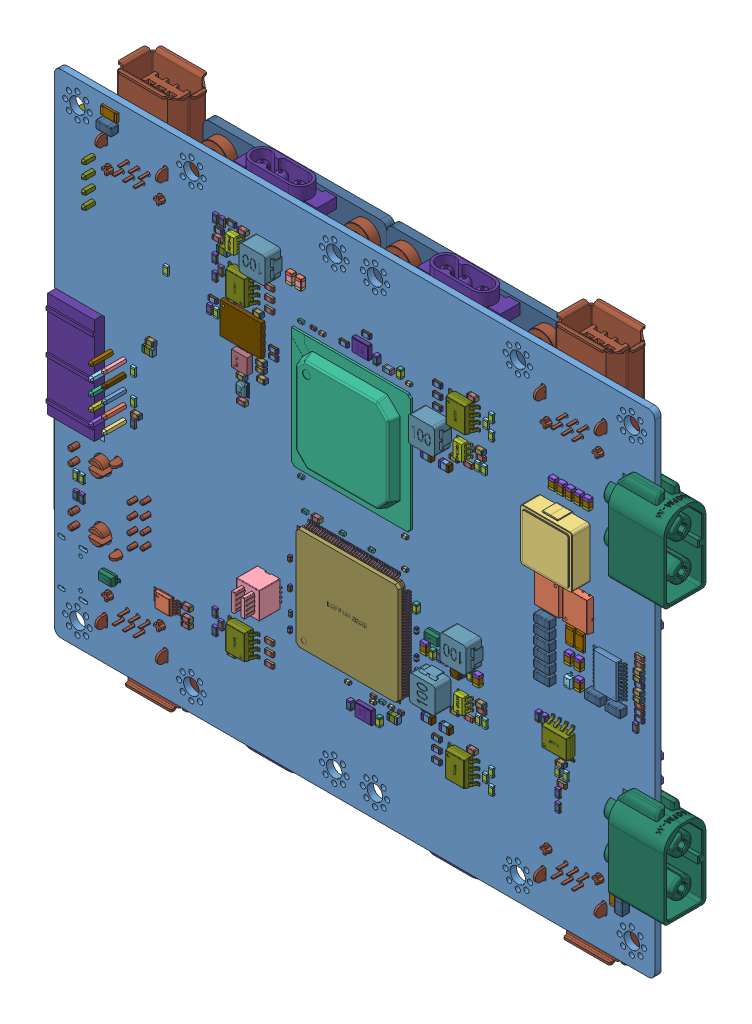
SolidWorks assembly Mother  Board, configuration 默认. Lengths in mm. (continued)
Components (placement in the parent): (continued)
- Mother  Board.step-1: Mother  Board.step [默认] at origin size (122.6 102.08 21) (continued)
  - C1_D4.step-1: C1_D4.step [默认] at origin size (1.6 0.8 0.8) (continued)
    - 5993854224.step-1: 5993854224.step [默认] at (76.6661 75.9461 0) x (1 0 0) z (0 0 1) size (1.6 0.8 0.8) (continued)
      - Terminal-17.step-1: Terminal-17.step [默认] at (-0.8 -0.4 0) size (1.6 0.8 0.8) (continued)
        - Open_CASCADE_STEP_translator_6.8_47.1.2-61.step-1: Open_CASCADE_STEP_translator_6.8_47.1.2-61.step [默认] at origin size (0.3 0.8 0.8)
      - Mid_Body-8.step-1: Mid_Body-8.step [默认] at (-0.8 -0.4 0) size (1 0.8 0.8)
        - Open_CASCADE_STEP_translator_6.8_47.2.1-62.step-1: Open_CASCADE_STEP_translator_6.8_47.2.1-62.step [默认] at origin size (1 0.8 0.8)
  - C1_D3.step-1: C1_D3.step [默认] at origin size (1.6 0.8 0.8)
    - 5993853264.step-1: 5993853264.step [默认] at (30.3949 69.2149 0) x (-1 0 0) z (0 0 1) size (1.6 0.8 0.8)
      - Terminal-6.step-1: Terminal-6.step [默认] at (-0.8 -0.4 0) size (1.6 0.8 0.8)
        - Open_CASCADE_STEP_translator_6.8_47.1.1-10.step-1: Open_CASCADE_STEP_translator_6.8_47.1.1-10.step [默认] at origin size (0.3 0.8 0.8)
        - Open_CASCADE_STEP_translator_6.8_47.1.2-11.step-1: Open_CASCADE_STEP_translator_6.8_47.1.2-11.step [默认] at origin size (0.3 0.8 0.8)
      - Mid_Body-5.step-1: Mid_Body-5.step [默认] at (-0.8 -0.4 0) size (1 0.8 0.8)
        - Open_CASCADE_STEP_translator_6.8_47.2.1-12.step-1: Open_CASCADE_STEP_translator_6.8_47.2.1-12.step [默认] at origin size (1 0.8 0.8)
  - C1_D2.step-1: C1_D2.step [默认] at origin size (1.6 0.8 0.8)
    - 5993854224.step-1: 5993854224.step [默认] at (76.5811 16.8911 0) x (1 0 0) z (0 0 1) size (1.6 0.8 0.8)
      - Terminal-17.step-1: Terminal-17.step [默认] at (-0.8 -0.4 0) size (1.6 0.8 0.8)
        - Open_CASCADE_STEP_translator_6.8_47.1.1-60.step-1: Open_CASCADE_STEP_translator_6.8_47.1.1-60.step [默认] at origin size (0.3 0.8 0.8)
        - Open_CASCADE_STEP_translator_6.8_47.1.2-61.step-1: Open_CASCADE_STEP_translator_6.8_47.1.2-61.step [默认] at origin size (0.3 0.8 0.8)
      - Mid_Body-8.step-1: Mid_Body-8.step [默认] at (-0.8 -0.4 0) size (1 0.8 0.8)
        - Open_CASCADE_STEP_translator_6.8_47.2.1-62.step-1: Open_CASCADE_STEP_translator_6.8_47.2.1-62.step [默认] at origin size (1 0.8 0.8)
  - C1_D1.step-1: C1_D1.step [默认] at origin size (1.6 0.8 0.8)
    - 5993853264.step-1: 5993853264.step [默认] at (30.3949 10.0329 0) x (-1 0 0) z (0 0 1) size (1.6 0.8 0.8)
      - Terminal-6.step-1: Terminal-6.step [默认] at (-0.8 -0.4 0) size (1.6 0.8 0.8)
        - Open_CASCADE_STEP_translator_6.8_47.1.1-10.step-1: Open_CASCADE_STEP_translator_6.8_47.1.1-10.step [默认] at origin size (0.3 0.8 0.8)
        - Open_CASCADE_STEP_translator_6.8_47.1.2-11.step-1: Open_CASCADE_STEP_translator_6.8_47.1.2-11.step [默认] at origin size (0.3 0.8 0.8)
      - Mid_Body-5.step-1: Mid_Body-5.step [默认] at (-0.8 -0.4 0) size (1 0.8 0.8)
        - Open_CASCADE_STEP_translator_6.8_47.2.1-12.step-1: Open_CASCADE_STEP_translator_6.8_47.2.1-12.step [默认] at origin size (1 0.8 0.8)
  - Free-Models.step-1: Free-Models.step [默认] at origin size (70.87 98.07 8.62)
    - Driver_Board.step-1: Driver_Board.step [默认] at (49.5407 86.106 -6.2) x (-1 0 0) z (0 0 1) size (35.43 49.03 8.62)
      - Board-1.step-1: Board-1.step [默认] at origin size (35.43 46.99 1.62)
        - Open_CASCADE_STEP_translator_6.8_2.1.1.step-1: Open_CASCADE_STEP_translator_6.8_2.1.1.step [默认] at (0 0 -1.6164) size (35.43 46.99 1.62)
      - R25-1.step-1: R25-1.step [默认] at origin size (0.8 1.6 0.45)
        - 6547515376.step-1: 6547515376.step [默认] at (20.6304 35.5601 0) x (0 1 0) z (0 0 1) size (1.6 0.8 0.45)
          - Terminal-19.step-1: Terminal-19.step [默认] at (-0.8 -0.4 0) size (0.3 0.8 0.45)
            - Open_CASCADE_STEP_translator_6.8_21.2.1-76.step-1: Open_CASCADE_STEP_translator_6.8_21.2.1-76.step [默认] at origin size (0.3 0.8 0.45)
          - Terminal-19.step-2: Terminal-19.step [默认] at (0.8 0.4 0) x (-1 0 0) z (0 0 1) size (0.3 0.8 0.45)
            - Open_CASCADE_STEP_translator_6.8_21.2.1-76.step-1: Open_CASCADE_STEP_translator_6.8_21.2.1-76.step [默认] at origin size (0.3 0.8 0.45)
          - Mid_Body-77.step-1: Mid_Body-77.step [默认] at (-0.8 -0.4 0) size (1.51 0.8 0.36)
          - Mark-78.step-1: Mark-78.step [默认] at (-0.5 -0.4 0.405) size (1 0.8 0.05)
      - R24-1.step-1: R24-1.step [默认] at origin size (1.6 0.8 0.45)
        - 6547516336.step-1: 6547516336.step [默认] at (12.6999 34.9249 0) x (-1 0 0) z (0 0 1) size (1.6 0.8 0.45)
          - Terminal-20.step-1: Terminal-20.step [默认] at (-0.8 -0.4 0) size (0.3 0.8 0.45)
            - Open_CASCADE_STEP_translator_6.8_21.2.1-79.step-1: Open_CASCADE_STEP_translator_6.8_21.2.1-79.step [默认] at origin size (0.3 0.8 0.45)
          - Terminal-20.step-2: Terminal-20.step [默认] at (0.8 0.4 0) x (-1 0 0) z (0 0 1) size (0.3 0.8 0.45)
            - Open_CASCADE_STEP_translator_6.8_21.2.1-79.step-1: Open_CASCADE_STEP_translator_6.8_21.2.1-79.step [默认] at origin size (0.3 0.8 0.45)
          - Mid_Body-80.step-1: Mid_Body-80.step [默认] at (-0.8 -0.4 0) size (1.51 0.8 0.36)
          - Mark-81.step-1: Mark-81.step [默认] at (-0.5 -0.4 0.405) size (1 0.8 0.05)
      - R23-1.step-1: R23-1.step [默认] at origin size (1.6 0.8 0.45)
        - 6547516336.step-1: 6547516336.step [默认] at (5.5879 33.6549 0) x (-1 0 0) z (0 0 1) size (1.6 0.8 0.45)
          - Terminal-20.step-1: Terminal-20.step [默认] at (-0.8 -0.4 0) size (0.3 0.8 0.45)
            - Open_CASCADE_STEP_translator_6.8_21.2.1-79.step-1: Open_CASCADE_STEP_translator_6.8_21.2.1-79.step [默认] at origin size (0.3 0.8 0.45)
          - Terminal-20.step-2: Terminal-20.step [默认] at (0.8 0.4 0) x (-1 0 0) z (0 0 1) size (0.3 0.8 0.45)
            - Open_CASCADE_STEP_translator_6.8_21.2.1-79.step-1: Open_CASCADE_STEP_translator_6.8_21.2.1-79.step [默认] at origin size (0.3 0.8 0.45)
          - Mid_Body-80.step-1: Mid_Body-80.step [默认] at (-0.8 -0.4 0) size (1.51 0.8 0.36)
          - Mark-81.step-1: Mark-81.step [默认] at (-0.5 -0.4 0.405) size (1 0.8 0.05)
      - JP1.step-1: JP1.step [默认] at origin size (16.01 14.49 6.96)
        - User_Library-MR30PW-M.step-1: User_Library-MR30PW-M.step [默认] at (13.7158 -5.9802 2.75) x (1 0 0) z (0 0 1) size (16.01 14.49 6.96)
      - R18-1.step-1: R18-1.step [默认] at origin size (0.8 1.6 0.45)
        - 6547515376.step-1: 6547515376.step [默认] at (22.9869 34.4171 0) x (0 1 0) z (0 0 1) size (1.6 0.8 0.45)
          - Terminal-19.step-1: Terminal-19.step [默认] at (-0.8 -0.4 0) size (0.3 0.8 0.45)
            - Open_CASCADE_STEP_translator_6.8_21.2.1-76.step-1: Open_CASCADE_STEP_translator_6.8_21.2.1-76.step [默认] at origin size (0.3 0.8 0.45)
          - Terminal-19.step-2: Terminal-19.step [默认] at (0.8 0.4 0) x (-1 0 0) z (0 0 1) size (0.3 0.8 0.45)
            - Open_CASCADE_STEP_translator_6.8_21.2.1-76.step-1: Open_CASCADE_STEP_translator_6.8_21.2.1-76.step [默认] at origin size (0.3 0.8 0.45)
          - Mid_Body-77.step-1: Mid_Body-77.step [默认] at (-0.8 -0.4 0) size (1.51 0.8 0.36)
          - Mark-78.step-1: Mark-78.step [默认] at (-0.5 -0.4 0.405) size (1 0.8 0.05)
      - R17-1.step-1: R17-1.step [默认] at origin size (0.8 1.6 0.45)
        - 6547515376.step-1: 6547515376.step [默认] at (21.8663 34.3947 0) x (0 1 0) z (0 0 1) size (1.6 0.8 0.45)
          - Terminal-19.step-1: Terminal-19.step [默认] at (-0.8 -0.4 0) size (0.3 0.8 0.45)
            - Open_CASCADE_STEP_translator_6.8_21.2.1-76.step-1: Open_CASCADE_STEP_translator_6.8_21.2.1-76.step [默认] at origin size (0.3 0.8 0.45)
          - Terminal-19.step-2: Terminal-19.step [默认] at (0.8 0.4 0) x (-1 0 0) z (0 0 1) size (0.3 0.8 0.45)
            - Open_CASCADE_STEP_translator_6.8_21.2.1-76.step-1: Open_CASCADE_STEP_translator_6.8_21.2.1-76.step [默认] at origin size (0.3 0.8 0.45)
          - Mid_Body-77.step-1: Mid_Body-77.step [默认] at (-0.8 -0.4 0) size (1.51 0.8 0.36)
          - Mark-78.step-1: Mark-78.step [默认] at (-0.5 -0.4 0.405) size (1 0.8 0.05)
      - R16-1.step-1: R16-1.step [默认] at origin size (1.6 0.8 0.45)
        - 6547506496.step-1: 6547506496.step [默认] at (16.6371 33.6551 0) x (1 0 0) z (0 0 1) size (1.6 0.8 0.45)
          - Terminal-21.step-1: Terminal-21.step [默认] at (-0.8 -0.4 0) size (0.3 0.8 0.45)
            - Open_CASCADE_STEP_translator_6.8_21.2.1-82.step-1: Open_CASCADE_STEP_translator_6.8_21.2.1-82.step [默认] at origin size (0.3 0.8 0.45)
          - Terminal-21.step-2: Terminal-21.step [默认] at (0.8 0.4 0) x (-1 0 0) z (0 0 1) size (0.3 0.8 0.45)
            - Open_CASCADE_STEP_translator_6.8_21.2.1-82.step-1: Open_CASCADE_STEP_translator_6.8_21.2.1-82.step [默认] at origin size (0.3 0.8 0.45)
          - Mid_Body-83.step-1: Mid_Body-83.step [默认] at (-0.8 -0.4 0) size (1.51 0.8 0.36)
          - Mark-84.step-1: Mark-84.step [默认] at (-0.5 -0.4 0.405) size (1 0.8 0.05)
      - R15-1.step-1: R15-1.step [默认] at origin size (0.8 1.6 0.45)
        - 6547515376.step-1: 6547515376.step [默认] at (14.7319 34.2901 0) x (0 1 0) z (0 0 1) size (1.6 0.8 0.45)
          - Terminal-19.step-1: Terminal-19.step [默认] at (-0.8 -0.4 0) size (0.3 0.8 0.45)
            - Open_CASCADE_STEP_translator_6.8_21.2.1-76.step-1: Open_CASCADE_STEP_translator_6.8_21.2.1-76.step [默认] at origin size (0.3 0.8 0.45)
          - Terminal-19.step-2: Terminal-19.step [默认] at (0.8 0.4 0) x (-1 0 0) z (0 0 1) size (0.3 0.8 0.45)
            - Open_CASCADE_STEP_translator_6.8_21.2.1-76.step-1: Open_CASCADE_STEP_translator_6.8_21.2.1-76.step [默认] at origin size (0.3 0.8 0.45)
          - Mid_Body-77.step-1: Mid_Body-77.step [默认] at (-0.8 -0.4 0) size (1.51 0.8 0.36)
          - Mark-78.step-1: Mark-78.step [默认] at (-0.5 -0.4 0.405) size (1 0.8 0.05)
      - R13-1.step-1: R13-1.step [默认] at origin size (1.6 0.8 0.45)
        - 6547506496.step-1: 6547506496.step [默认] at (9.5251 33.6551 0) x (1 0 0) z (0 0 1) size (1.6 0.8 0.45)
          - Terminal-21.step-1: Terminal-21.step [默认] at (-0.8 -0.4 0) size (0.3 0.8 0.45)
            - Open_CASCADE_STEP_translator_6.8_21.2.1-82.step-1: Open_CASCADE_STEP_translator_6.8_21.2.1-82.step [默认] at origin size (0.3 0.8 0.45)
          - Terminal-21.step-2: Terminal-21.step [默认] at (0.8 0.4 0) x (-1 0 0) z (0 0 1) size (0.3 0.8 0.45)
            - Open_CASCADE_STEP_translator_6.8_21.2.1-82.step-1: Open_CASCADE_STEP_translator_6.8_21.2.1-82.step [默认] at origin size (0.3 0.8 0.45)
          - Mid_Body-83.step-1: Mid_Body-83.step [默认] at (-0.8 -0.4 0) size (1.51 0.8 0.36)
          - Mark-84.step-1: Mark-84.step [默认] at (-0.5 -0.4 0.405) size (1 0.8 0.05)
      - R11-1.step-1: R11-1.step [默认] at origin size (0.8 1.6 0.45)
        - 6547515376.step-1: 6547515376.step [默认] at (7.6423 34.2901 0) x (0 1 0) z (0 0 1) size (1.6 0.8 0.45)
          - Terminal-19.step-1: Terminal-19.step [默认] at (-0.8 -0.4 0) size (0.3 0.8 0.45)
            - Open_CASCADE_STEP_translator_6.8_21.2.1-76.step-1: Open_CASCADE_STEP_translator_6.8_21.2.1-76.step [默认] at origin size (0.3 0.8 0.45)
          - Terminal-19.step-2: Terminal-19.step [默认] at (0.8 0.4 0) x (-1 0 0) z (0 0 1) size (0.3 0.8 0.45)
            - Open_CASCADE_STEP_translator_6.8_21.2.1-76.step-1: Open_CASCADE_STEP_translator_6.8_21.2.1-76.step [默认] at origin size (0.3 0.8 0.45)
          - Mid_Body-77.step-1: Mid_Body-77.step [默认] at (-0.8 -0.4 0) size (1.51 0.8 0.36)
          - Mark-78.step-1: Mark-78.step [默认] at (-0.5 -0.4 0.405) size (1 0.8 0.05)
      - C23-1.step-1: C23-1.step [默认] at origin size (1.6 0.8 0.8)
        - 6547515616.step-1: 6547515616.step [默认] at (19.8684 33.6676 0) x (-1 0 0) z (0 0 1) size (1.6 0.8 0.8)
          - Terminal-22.step-1: Terminal-22.step [默认] at (-0.8 -0.4 0) size (1.6 0.8 0.8)
            - Open_CASCADE_STEP_translator_6.8_47.1.1-85.step-1: Open_CASCADE_STEP_translator_6.8_47.1.1-85.step [默认] at origin size (0.3 0.8 0.8)
            - Open_CASCADE_STEP_translator_6.8_47.1.2-86.step-1: Open_CASCADE_STEP_translator_6.8_47.1.2-86.step [默认] at origin size (0.3 0.8 0.8)
          - Mid_Body-10.step-1: Mid_Body-10.step [默认] at (-0.8 -0.4 0) size (1 0.8 0.8)
            - Open_CASCADE_STEP_translator_6.8_47.2.1-87.step-1: Open_CASCADE_STEP_translator_6.8_47.2.1-87.step [默认] at origin size (1 0.8 0.8)
      - C22-1.step-1: C22-1.step [默认] at origin size (1.6 0.8 0.8)
        - 6547515616.step-1: 6547515616.step [默认] at (12.6999 33.6549 0) x (-1 0 0) z (0 0 1) size (1.6 0.8 0.8)
          - Terminal-22.step-1: Terminal-22.step [默认] at (-0.8 -0.4 0) size (1.6 0.8 0.8)
            - Open_CASCADE_STEP_translator_6.8_47.1.1-85.step-1: Open_CASCADE_STEP_translator_6.8_47.1.1-85.step [默认] at origin size (0.3 0.8 0.8)
            - Open_CASCADE_STEP_translator_6.8_47.1.2-86.step-1: Open_CASCADE_STEP_translator_6.8_47.1.2-86.step [默认] at origin size (0.3 0.8 0.8)
          - Mid_Body-10.step-1: Mid_Body-10.step [默认] at (-0.8 -0.4 0) size (1 0.8 0.8)
            - Open_CASCADE_STEP_translator_6.8_47.2.1-87.step-1: Open_CASCADE_STEP_translator_6.8_47.2.1-87.step [默认] at origin size (1 0.8 0.8)
      - C21-1.step-1: C21-1.step [默认] at origin size (1.6 0.8 0.8)
        - 6547515616.step-1: 6547515616.step [默认] at (5.6103 34.9025 0) x (-1 0 0) z (0 0 1) size (1.6 0.8 0.8)
          - Terminal-22.step-1: Terminal-22.step [默认] at (-0.8 -0.4 0) size (1.6 0.8 0.8)
            - Open_CASCADE_STEP_translator_6.8_47.1.1-85.step-1: Open_CASCADE_STEP_translator_6.8_47.1.1-85.step [默认] at origin size (0.3 0.8 0.8)
            - Open_CASCADE_STEP_translator_6.8_47.1.2-86.step-1: Open_CASCADE_STEP_translator_6.8_47.1.2-86.step [默认] at origin size (0.3 0.8 0.8)
          - Mid_Body-10.step-1: Mid_Body-10.step [默认] at (-0.8 -0.4 0) size (1 0.8 0.8)
            - Open_CASCADE_STEP_translator_6.8_47.2.1-87.step-1: Open_CASCADE_STEP_translator_6.8_47.2.1-87.step [默认] at origin size (1 0.8 0.8)
      - U5-1.step-1: U5-1.step [默认] at origin size (5.9 11.5 2.7)
        - SO8_W.step-1: SO8_W.step [默认] at (27.6859 29.9721 0.381) x (0 1 0) z (0 0 1) size (11.5 5.9 2.7)
      - U4-1.step-1: U4-1.step [默认] at origin size (5.9 11.5 2.7)
        - SO8_W.step-1: SO8_W.step [默认] at (-0.1271 29.9721 0.381) x (0 1 0) z (0 0 1) size (11.5 5.9 2.7)
      - U3-1.step-1: U3-1.step [默认] at origin size (5 6.01 1.9)
        - SOP8-1.step-1: SOP8-1.step [默认] at (19.9615 29.5285 0) x (0 -1 0) z (0 0 1) size (6.01 5 1.9)
          - LOGO_-88.step-1: LOGO_-88.step [默认] at (0.0116 0 0.095) x (0 -1 0) z (0 0 -1) size (1.5 1.73 0.01)
          - SOP8-89.step-1: SOP8-89.step [默认] at origin size (6.01 5 1.9)
      - U2-1.step-1: U2-1.step [默认] at origin size (5 6.01 1.9)
        - SOP8-1.step-1: SOP8-1.step [默认] at (12.8495 29.5285 0) x (0 -1 0) z (0 0 1) size (6.01 5 1.9)
          - LOGO_-88.step-1: LOGO_-88.step [默认] at (0.0116 0 0.095) x (0 -1 0) z (0 0 -1) size (1.5 1.73 0.01)
          - SOP8-89.step-1: SOP8-89.step [默认] at origin size (6.01 5 1.9)
      - U1.step-1: U1.step [默认] at origin size (5 6.01 1.9)
        - SOP8-1.step-1: SOP8-1.step [默认] at (5.7375 29.5285 0) x (0 -1 0) z (0 0 1) size (6.01 5 1.9)
          - LOGO_-88.step-1: LOGO_-88.step [默认] at (0.0116 0 0.095) x (0 -1 0) z (0 0 -1) size (1.5 1.73 0.01)
          - SOP8-89.step-1: SOP8-89.step [默认] at origin size (6.01 5 1.9)
      - RS2-1.step-1: RS2-1.step [默认] at origin size (3.1 1.55 0.47)
        - User_Library-R1206-90.step-1: User_Library-R1206-90.step [默认] at (23.7489 17.5261 -1.6164) x (-1 0 0) z (0 0 -1) size (3.1 1.55 0.47)
      - RS1-1.step-1: RS1-1.step [默认] at origin size (3.1 1.55 0.47)
        - User_Library-R1206-90.step-1: User_Library-R1206-90.step [默认] at (-0.1271 18.1611 -1.6164) x (-1 0 0) z (0 0 -1) size (3.1 1.55 0.47)
      - R22-1.step-1: R22-1.step [默认] at origin size (1.6 0.8 0.45)
        - 6547506496.step-1: 6547506496.step [默认] at (22.9871 17.7801 0) x (1 0 0) z (0 0 1) size (1.6 0.8 0.45)
          - Terminal-21.step-1: Terminal-21.step [默认] at (-0.8 -0.4 0) size (0.3 0.8 0.45)
            - Open_CASCADE_STEP_translator_6.8_21.2.1-82.step-1: Open_CASCADE_STEP_translator_6.8_21.2.1-82.step [默认] at origin size (0.3 0.8 0.45)
          - Terminal-21.step-2: Terminal-21.step [默认] at (0.8 0.4 0) x (-1 0 0) z (0 0 1) size (0.3 0.8 0.45)
            - Open_CASCADE_STEP_translator_6.8_21.2.1-82.step-1: Open_CASCADE_STEP_translator_6.8_21.2.1-82.step [默认] at origin size (0.3 0.8 0.45)
          - Mid_Body-83.step-1: Mid_Body-83.step [默认] at (-0.8 -0.4 0) size (1.51 0.8 0.36)
          - Mark-84.step-1: Mark-84.step [默认] at (-0.5 -0.4 0.405) size (1 0.8 0.05)
      - R21-1.step-1: R21-1.step [默认] at origin size (1.6 0.8 0.45)
        - 6547516336.step-1: 6547516336.step [默认] at (22.9869 18.9229 0) x (-1 0 0) z (0 0 1) size (1.6 0.8 0.45)
          - Terminal-20.step-1: Terminal-20.step [默认] at (-0.8 -0.4 0) size (0.3 0.8 0.45)
            - Open_CASCADE_STEP_translator_6.8_21.2.1-79.step-1: Open_CASCADE_STEP_translator_6.8_21.2.1-79.step [默认] at origin size (0.3 0.8 0.45)
          - Terminal-20.step-2: Terminal-20.step [默认] at (0.8 0.4 0) x (-1 0 0) z (0 0 1) size (0.3 0.8 0.45)
            - Open_CASCADE_STEP_translator_6.8_21.2.1-79.step-1: Open_CASCADE_STEP_translator_6.8_21.2.1-79.step [默认] at origin size (0.3 0.8 0.45)
          - Mid_Body-80.step-1: Mid_Body-80.step [默认] at (-0.8 -0.4 0) size (1.51 0.8 0.36)
          - Mark-81.step-1: Mark-81.step [默认] at (-0.5 -0.4 0.405) size (1 0.8 0.05)
      - R20-1.step-1: R20-1.step [默认] at origin size (1.6 0.8 0.45)
        - 6547506496.step-1: 6547506496.step [默认] at (24.6381 11.8111 0) x (1 0 0) z (0 0 1) size (1.6 0.8 0.45)
          - Terminal-21.step-1: Terminal-21.step [默认] at (-0.8 -0.4 0) size (0.3 0.8 0.45)
            - Open_CASCADE_STEP_translator_6.8_21.2.1-82.step-1: Open_CASCADE_STEP_translator_6.8_21.2.1-82.step [默认] at origin size (0.3 0.8 0.45)
          - Terminal-21.step-2: Terminal-21.step [默认] at (0.8 0.4 0) x (-1 0 0) z (0 0 1) size (0.3 0.8 0.45)
            - Open_CASCADE_STEP_translator_6.8_21.2.1-82.step-1: Open_CASCADE_STEP_translator_6.8_21.2.1-82.step [默认] at origin size (0.3 0.8 0.45)
          - Mid_Body-83.step-1: Mid_Body-83.step [默认] at (-0.8 -0.4 0) size (1.51 0.8 0.36)
          - Mark-84.step-1: Mark-84.step [默认] at (-0.5 -0.4 0.405) size (1 0.8 0.05)
      - R19-1.step-1: R19-1.step [默认] at origin size (0.8 1.6 0.45)
        - 6547515376.step-1: 6547515376.step [默认] at (25.3999 13.5891 0) x (0 1 0) z (0 0 1) size (1.6 0.8 0.45)
          - Terminal-19.step-1: Terminal-19.step [默认] at (-0.8 -0.4 0) size (0.3 0.8 0.45)
            - Open_CASCADE_STEP_translator_6.8_21.2.1-76.step-1: Open_CASCADE_STEP_translator_6.8_21.2.1-76.step [默认] at origin size (0.3 0.8 0.45)
          - Terminal-19.step-2: Terminal-19.step [默认] at (0.8 0.4 0) x (-1 0 0) z (0 0 1) size (0.3 0.8 0.45)
            - Open_CASCADE_STEP_translator_6.8_21.2.1-76.step-1: Open_CASCADE_STEP_translator_6.8_21.2.1-76.step [默认] at origin size (0.3 0.8 0.45)
          - Mid_Body-77.step-1: Mid_Body-77.step [默认] at (-0.8 -0.4 0) size (1.51 0.8 0.36)
          - Mark-78.step-1: Mark-78.step [默认] at (-0.5 -0.4 0.405) size (1 0.8 0.05)
      - R14-1.step-1: R14-1.step [默认] at origin size (1.6 0.8 0.45)
        - 6547506496.step-1: 6547506496.step [默认] at (12.0651 20.0661 0) x (1 0 0) z (0 0 1) size (1.6 0.8 0.45)
          - Terminal-21.step-1: Terminal-21.step [默认] at (-0.8 -0.4 0) size (0.3 0.8 0.45)
            - Open_CASCADE_STEP_translator_6.8_21.2.1-82.step-1: Open_CASCADE_STEP_translator_6.8_21.2.1-82.step [默认] at origin size (0.3 0.8 0.45)
          - Terminal-21.step-2: Terminal-21.step [默认] at (0.8 0.4 0) x (-1 0 0) z (0 0 1) size (0.3 0.8 0.45)
            - Open_CASCADE_STEP_translator_6.8_21.2.1-82.step-1: Open_CASCADE_STEP_translator_6.8_21.2.1-82.step [默认] at origin size (0.3 0.8 0.45)
          - Mid_Body-83.step-1: Mid_Body-83.step [默认] at (-0.8 -0.4 0) size (1.51 0.8 0.36)
          - Mark-84.step-1: Mark-84.step [默认] at (-0.5 -0.4 0.405) size (1 0.8 0.05)
      - R12-1.step-1: R12-1.step [默认] at origin size (1.6 0.8 0.45)
        - 6547516336.step-1: 6547516336.step [默认] at (12.0649 21.2089 0) x (-1 0 0) z (0 0 1) size (1.6 0.8 0.45)
          - Terminal-20.step-1: Terminal-20.step [默认] at (-0.8 -0.4 0) size (0.3 0.8 0.45)
            - Open_CASCADE_STEP_translator_6.8_21.2.1-79.step-1: Open_CASCADE_STEP_translator_6.8_21.2.1-79.step [默认] at origin size (0.3 0.8 0.45)
          - Terminal-20.step-2: Terminal-20.step [默认] at (0.8 0.4 0) x (-1 0 0) z (0 0 1) size (0.3 0.8 0.45)
            - Open_CASCADE_STEP_translator_6.8_21.2.1-79.step-1: Open_CASCADE_STEP_translator_6.8_21.2.1-79.step [默认] at origin size (0.3 0.8 0.45)
          - Mid_Body-80.step-1: Mid_Body-80.step [默认] at (-0.8 -0.4 0) size (1.51 0.8 0.36)
          - Mark-81.step-1: Mark-81.step [默认] at (-0.5 -0.4 0.405) size (1 0.8 0.05)
      - R10-1.step-1: R10-1.step [默认] at origin size (1.6 0.8 0.45)
        - 6547506496.step-1: 6547506496.step [默认] at (13.7161 14.0971 0) x (1 0 0) z (0 0 1) size (1.6 0.8 0.45)
          - Terminal-21.step-1: Terminal-21.step [默认] at (-0.8 -0.4 0) size (0.3 0.8 0.45)
            - Open_CASCADE_STEP_translator_6.8_21.2.1-82.step-1: Open_CASCADE_STEP_translator_6.8_21.2.1-82.step [默认] at origin size (0.3 0.8 0.45)
          - Terminal-21.step-2: Terminal-21.step [默认] at (0.8 0.4 0) x (-1 0 0) z (0 0 1) size (0.3 0.8 0.45)
            - Open_CASCADE_STEP_translator_6.8_21.2.1-82.step-1: Open_CASCADE_STEP_translator_6.8_21.2.1-82.step [默认] at origin size (0.3 0.8 0.45)
          - Mid_Body-83.step-1: Mid_Body-83.step [默认] at (-0.8 -0.4 0) size (1.51 0.8 0.36)
          - Mark-84.step-1: Mark-84.step [默认] at (-0.5 -0.4 0.405) size (1 0.8 0.05)
      - R9-1.step-1: R9-1.step [默认] at origin size (0.8 1.6 0.45)
        - 6547515376.step-1: 6547515376.step [默认] at (14.4779 15.8751 0) x (0 1 0) z (0 0 1) size (1.6 0.8 0.45)
          - Terminal-19.step-1: Terminal-19.step [默认] at (-0.8 -0.4 0) size (0.3 0.8 0.45)
            - Open_CASCADE_STEP_translator_6.8_21.2.1-76.step-1: Open_CASCADE_STEP_translator_6.8_21.2.1-76.step [默认] at origin size (0.3 0.8 0.45)
          - Terminal-19.step-2: Terminal-19.step [默认] at (0.8 0.4 0) x (-1 0 0) z (0 0 1) size (0.3 0.8 0.45)
            - Open_CASCADE_STEP_translator_6.8_21.2.1-76.step-1: Open_CASCADE_STEP_translator_6.8_21.2.1-76.step [默认] at origin size (0.3 0.8 0.45)
          - Mid_Body-77.step-1: Mid_Body-77.step [默认] at (-0.8 -0.4 0) size (1.51 0.8 0.36)
          - Mark-78.step-1: Mark-78.step [默认] at (-0.5 -0.4 0.405) size (1 0.8 0.05)
      - R8-1.step-1: R8-1.step [默认] at origin size (0.8 1.6 0.45)
        - 6547515376.step-1: 6547515376.step [默认] at (28.3209 21.0821 0) x (0 1 0) z (0 0 1) size (1.6 0.8 0.45)
          - Terminal-19.step-1: Terminal-19.step [默认] at (-0.8 -0.4 0) size (0.3 0.8 0.45)
            - Open_CASCADE_STEP_translator_6.8_21.2.1-76.step-1: Open_CASCADE_STEP_translator_6.8_21.2.1-76.step [默认] at origin size (0.3 0.8 0.45)
          - Terminal-19.step-2: Terminal-19.step [默认] at (0.8 0.4 0) x (-1 0 0) z (0 0 1) size (0.3 0.8 0.45)
            - Open_CASCADE_STEP_translator_6.8_21.2.1-76.step-1: Open_CASCADE_STEP_translator_6.8_21.2.1-76.step [默认] at origin size (0.3 0.8 0.45)
          - Mid_Body-77.step-1: Mid_Body-77.step [默认] at (-0.8 -0.4 0) size (1.51 0.8 0.36)
          - Mark-78.step-1: Mark-78.step [默认] at (-0.5 -0.4 0.405) size (1 0.8 0.05)
      - R7-1.step-1: R7-1.step [默认] at origin size (0.8 1.6 0.45)
        - 6547515376.step-1: 6547515376.step [默认] at (27.0509 21.0821 0) x (0 1 0) z (0 0 1) size (1.6 0.8 0.45)
          - Terminal-19.step-1: Terminal-19.step [默认] at (-0.8 -0.4 0) size (0.3 0.8 0.45)
            - Open_CASCADE_STEP_translator_6.8_21.2.1-76.step-1: Open_CASCADE_STEP_translator_6.8_21.2.1-76.step [默认] at origin size (0.3 0.8 0.45)
          - Terminal-19.step-2: Terminal-19.step [默认] at (0.8 0.4 0) x (-1 0 0) z (0 0 1) size (0.3 0.8 0.45)
            - Open_CASCADE_STEP_translator_6.8_21.2.1-76.step-1: Open_CASCADE_STEP_translator_6.8_21.2.1-76.step [默认] at origin size (0.3 0.8 0.45)
          - Mid_Body-77.step-1: Mid_Body-77.step [默认] at (-0.8 -0.4 0) size (1.51 0.8 0.36)
          - Mark-78.step-1: Mark-78.step [默认] at (-0.5 -0.4 0.405) size (1 0.8 0.05)
      - R6.step-1: R6.step [默认] at origin size (1.6 0.8 0.45)
        - 6547506496.step-1: 6547506496.step [默认] at (1.1431 17.6531 0) x (1 0 0) z (0 0 1) size (1.6 0.8 0.45)
          - Terminal-21.step-1: Terminal-21.step [默认] at (-0.8 -0.4 0) size (0.3 0.8 0.45)
            - Open_CASCADE_STEP_translator_6.8_21.2.1-82.step-1: Open_CASCADE_STEP_translator_6.8_21.2.1-82.step [默认] at origin size (0.3 0.8 0.45)
          - Terminal-21.step-2: Terminal-21.step [默认] at (0.8 0.4 0) x (-1 0 0) z (0 0 1) size (0.3 0.8 0.45)
            - Open_CASCADE_STEP_translator_6.8_21.2.1-82.step-1: Open_CASCADE_STEP_translator_6.8_21.2.1-82.step [默认] at origin size (0.3 0.8 0.45)
          - Mid_Body-83.step-1: Mid_Body-83.step [默认] at (-0.8 -0.4 0) size (1.51 0.8 0.36)
          - Mark-84.step-1: Mark-84.step [默认] at (-0.5 -0.4 0.405) size (1 0.8 0.05)
      - R5.step-1: R5.step [默认] at origin size (0.8 1.6 0.45)
        - 6547515376.step-1: 6547515376.step [默认] at (1.7779 21.0821 0) x (0 1 0) z (0 0 1) size (1.6 0.8 0.45)
          - Terminal-19.step-1: Terminal-19.step [默认] at (-0.8 -0.4 0) size (0.3 0.8 0.45)
            - Open_CASCADE_STEP_translator_6.8_21.2.1-76.step-1: Open_CASCADE_STEP_translator_6.8_21.2.1-76.step [默认] at origin size (0.3 0.8 0.45)
          - Terminal-19.step-2: Terminal-19.step [默认] at (0.8 0.4 0) x (-1 0 0) z (0 0 1) size (0.3 0.8 0.45)
            - Open_CASCADE_STEP_translator_6.8_21.2.1-76.step-1: Open_CASCADE_STEP_translator_6.8_21.2.1-76.step [默认] at origin size (0.3 0.8 0.45)
          - Mid_Body-77.step-1: Mid_Body-77.step [默认] at (-0.8 -0.4 0) size (1.51 0.8 0.36)
          - Mark-78.step-1: Mark-78.step [默认] at (-0.5 -0.4 0.405) size (1 0.8 0.05)
      - R4.step-1: R4.step [默认] at origin size (0.8 1.6 0.45)
        - 6547515376.step-1: 6547515376.step [默认] at (0.5079 21.0821 0) x (0 1 0) z (0 0 1) size (1.6 0.8 0.45)
          - Terminal-19.step-1: Terminal-19.step [默认] at (-0.8 -0.4 0) size (0.3 0.8 0.45)
            - Open_CASCADE_STEP_translator_6.8_21.2.1-76.step-1: Open_CASCADE_STEP_translator_6.8_21.2.1-76.step [默认] at origin size (0.3 0.8 0.45)
          - Terminal-19.step-2: Terminal-19.step [默认] at (0.8 0.4 0) x (-1 0 0) z (0 0 1) size (0.3 0.8 0.45)
            - Open_CASCADE_STEP_translator_6.8_21.2.1-76.step-1: Open_CASCADE_STEP_translator_6.8_21.2.1-76.step [默认] at origin size (0.3 0.8 0.45)
          - Mid_Body-77.step-1: Mid_Body-77.step [默认] at (-0.8 -0.4 0) size (1.51 0.8 0.36)
          - Mark-78.step-1: Mark-78.step [默认] at (-0.5 -0.4 0.405) size (1 0.8 0.05)
      - R3.step-1: R3.step [默认] at origin size (1.6 0.8 0.45)
        - 6547506496.step-1: 6547506496.step [默认] at (2.7941 11.8111 0) x (1 0 0) z (0 0 1) size (1.6 0.8 0.45)
          - Terminal-21.step-1: Terminal-21.step [默认] at (-0.8 -0.4 0) size (0.3 0.8 0.45)
            - Open_CASCADE_STEP_translator_6.8_21.2.1-82.step-1: Open_CASCADE_STEP_translator_6.8_21.2.1-82.step [默认] at origin size (0.3 0.8 0.45)
          - Terminal-21.step-2: Terminal-21.step [默认] at (0.8 0.4 0) x (-1 0 0) z (0 0 1) size (0.3 0.8 0.45)
            - Open_CASCADE_STEP_translator_6.8_21.2.1-82.step-1: Open_CASCADE_STEP_translator_6.8_21.2.1-82.step [默认] at origin size (0.3 0.8 0.45)
          - Mid_Body-83.step-1: Mid_Body-83.step [默认] at (-0.8 -0.4 0) size (1.51 0.8 0.36)
          - Mark-84.step-1: Mark-84.step [默认] at (-0.5 -0.4 0.405) size (1 0.8 0.05)
      - R2.step-1: R2.step [默认] at origin size (0.8 1.6 0.45)
        - 6547515376.step-1: 6547515376.step [默认] at (-0.7621 21.0821 0) x (0 1 0) z (0 0 1) size (1.6 0.8 0.45)
          - Terminal-19.step-1: Terminal-19.step [默认] at (-0.8 -0.4 0) size (0.3 0.8 0.45)
            - Open_CASCADE_STEP_translator_6.8_21.2.1-76.step-1: Open_CASCADE_STEP_translator_6.8_21.2.1-76.step [默认] at origin size (0.3 0.8 0.45)
          - Terminal-19.step-2: Terminal-19.step [默认] at (0.8 0.4 0) x (-1 0 0) z (0 0 1) size (0.3 0.8 0.45)
            - Open_CASCADE_STEP_translator_6.8_21.2.1-76.step-1: Open_CASCADE_STEP_translator_6.8_21.2.1-76.step [默认] at origin size (0.3 0.8 0.45)
          - Mid_Body-77.step-1: Mid_Body-77.step [默认] at (-0.8 -0.4 0) size (1.51 0.8 0.36)
          - Mark-78.step-1: Mark-78.step [默认] at (-0.5 -0.4 0.405) size (1 0.8 0.05)
      - R1.step-1: R1.step [默认] at origin size (0.8 1.6 0.45)
        - 6547515376.step-1: 6547515376.step [默认] at (3.5559 13.5891 0) x (0 1 0) z (0 0 1) size (1.6 0.8 0.45)
          - Terminal-19.step-1: Terminal-19.step [默认] at (-0.8 -0.4 0) size (0.3 0.8 0.45)
            - Open_CASCADE_STEP_translator_6.8_21.2.1-76.step-1: Open_CASCADE_STEP_translator_6.8_21.2.1-76.step [默认] at origin size (0.3 0.8 0.45)
          - Terminal-19.step-2: Terminal-19.step [默认] at (0.8 0.4 0) x (-1 0 0) z (0 0 1) size (0.3 0.8 0.45)
            - Open_CASCADE_STEP_translator_6.8_21.2.1-76.step-1: Open_CASCADE_STEP_translator_6.8_21.2.1-76.step [默认] at origin size (0.3 0.8 0.45)
          - Mid_Body-77.step-1: Mid_Body-77.step [默认] at (-0.8 -0.4 0) size (1.51 0.8 0.36)
          - Mark-78.step-1: Mark-78.step [默认] at (-0.5 -0.4 0.405) size (1 0.8 0.05)
      - M6.step-1: M6.step [默认] at origin size (5.15 6.15 1.1)
        - TDSON-8-91.step-1: TDSON-8-91.step [默认] at (21.8441 12.7711 -1.6164) x (1 0 0) z (0 1 0) size (5.15 1.1 6.15)
      - M5.step-1: M5.step [默认] at origin size (5.15 6.15 1.1)
        - TDSON-8-91.step-1: TDSON-8-91.step [默认] at (27.3049 12.7713 -1.6164) x (-1 0 0) z (0 -1 0) size (5.15 1.1 6.15)
      - M4.step-1: M4.step [默认] at origin size (5.15 6.15 1.1)
        - TDSON-8-91.step-1: TDSON-8-91.step [默认] at (10.9221 15.0571 -1.6164) x (1 0 0) z (0 1 0) size (5.15 1.1 6.15)
      - M3.step-1: M3.step [默认] at origin size (5.15 6.15 1.1)
        - TDSON-8-91.step-1: TDSON-8-91.step [默认] at (16.3829 15.0573 -1.6164) x (-1 0 0) z (0 -1 0) size (5.15 1.1 6.15)
      - M2-1.step-1: M2-1.step [默认] at origin size (5.15 6.15 1.1)
        - TDSON-8-91.step-1: TDSON-8-91.step [默认] at (0 12.7711 -1.6164) x (1 0 0) z (0 1 0) size (5.15 1.1 6.15)
      - M1-1.step-1: M1-1.step [默认] at origin size (5.15 6.15 1.1)
        - TDSON-8-91.step-1: TDSON-8-91.step [默认] at (5.4609 12.7713 -1.6164) x (-1 0 0) z (0 -1 0) size (5.15 1.1 6.15)
      - JP4-1.step-1: JP4-1.step [默认] at origin size (5.56 5.56 4.53)
        - User_Library-SMTSO-M3-3ET.step-1: User_Library-SMTSO-M3-3ET.step [默认] at (27.5589 0.0001 -2.6164) x (0 0 1) z (0 1 0) size (4.53 5.56 5.56)
      - JP3-1.step-1: JP3-1.step [默认] at origin size (5.56 5.56 4.53)
        - User_Library-SMTSO-M3-3ET.step-1: User_Library-SMTSO-M3-3ET.step [默认] at (-0.0001 0.0001 -2.6164) x (0 0 1) z (0 1 0) size (4.53 5.56 5.56)
      - JP2.step-1: JP2.step [默认] at origin size (11.5 4.96 6.5)
        - SG340-GxxP-B1-2x12.step-1: SG340-GxxP-B1-2x12.step [默认] at (13.7793 38.9891 0) x (-1 0 0) z (0 0 1) size (11.5 4.96 6.5)
      - D3-1.step-1: D3-1.step [默认] at origin size (2.65 1.3 0.96)
        - SOD-323-1.step-1: SOD-323-1.step [默认] at (20.5836 25.1426 0.05) x (-1 0 0) z (0 0 1) size (2.65 1.3 0.96)
          - SOD-323-92.step-1: SOD-323-92.step [默认] at origin size (2.65 1.3 0.95)
          - LOGO______.__-93.step-1: LOGO______.__-93.step [默认] at (0.0033 0.0815 -0.003) x (-1 0 0) z (0 0 -1) size (0.9 1.04 0.01)
      - D2-1.step-1: D2-1.step [默认] at origin size (2.65 1.3 0.96)
        - SOD-323-1.step-1: SOD-323-1.step [默认] at (13.4716 25.1426 0.05) x (-1 0 0) z (0 0 1) size (2.65 1.3 0.96)
          - SOD-323-92.step-1: SOD-323-92.step [默认] at origin size (2.65 1.3 0.95)
          - LOGO______.__-93.step-1: LOGO______.__-93.step [默认] at (0.0033 0.0815 -0.003) x (-1 0 0) z (0 0 -1) size (0.9 1.04 0.01)
      - D1-1.step-1: D1-1.step [默认] at origin size (2.65 1.3 0.96)
        - SOD-323-1.step-1: SOD-323-1.step [默认] at (6.3596 25.1426 0.05) x (-1 0 0) z (0 0 1) size (2.65 1.3 0.96)
          - SOD-323-92.step-1: SOD-323-92.step [默认] at origin size (2.65 1.3 0.95)
          - LOGO______.__-93.step-1: LOGO______.__-93.step [默认] at (0.0033 0.0815 -0.003) x (-1 0 0) z (0 0 -1) size (0.9 1.04 0.01)
      - CP7-1.step-1: CP7-1.step [默认] at origin size (1.5 3 1.5)
        - (______)-94.step-1: (______)-94.step [默认] at (29.2101 17.1449 0) x (1 0 0) z (0 0 1) size (1.5 3 1.5)
      - CP9.step-1: CP9.step [默认] at origin size (1.5 3 1.5)
        - (______)-94.step-1: (______)-94.step [默认] at (18.2881 19.4309 0) x (1 0 0) z (0 0 1) size (1.5 3 1.5)
      - CP8-1.step-1: CP8-1.step [默认] at origin size (1.5 3 1.5)
        - (______)-94.step-1: (______)-94.step [默认] at (20.1931 19.4309 0) x (1 0 0) z (0 0 1) size (1.5 3 1.5)
      - CP5-1.step-1: CP5-1.step [默认] at origin size (1.5 3 1.5)
        - (______)-94.step-1: (______)-94.step [默认] at (9.3982 17.145 0) x (1 0 0) z (0 0 1) size (1.5 3 1.5)
      - CP4-1.step-1: CP4-1.step [默认] at origin size (1.5 3 1.5)
        - (______)-94.step-1: (______)-94.step [默认] at (7.4932 17.145 0) x (1 0 0) z (0 0 1) size (1.5 3 1.5)
      - CP3-1.step-1: CP3-1.step [默认] at origin size (1.5 3 1.5)
        - (______)-94.step-1: (______)-94.step [默认] at (27.3051 17.1449 0) x (1 0 0) z (0 0 1) size (1.5 3 1.5)
      - CP2-1.step-1: CP2-1.step [默认] at origin size (1.5 3 1.5)
        - (______)-94.step-1: (______)-94.step [默认] at (16.3831 19.4309 0) x (1 0 0) z (0 0 1) size (1.5 3 1.5)
      - CP1-1.step-1: CP1-1.step [默认] at origin size (1.5 3 1.5)
        - (______)-94.step-1: (______)-94.step [默认] at (5.5882 17.145 0) x (1 0 0) z (0 0 1) size (1.5 3 1.5)
      - C29-1.step-1: C29-1.step [默认] at origin size (1.6 0.8 0.8)
        - 6547515616.step-1: 6547515616.step [默认] at (22.9869 16.6369 0) x (-1 0 0) z (0 0 1) size (1.6 0.8 0.8)
          - Terminal-22.step-1: Terminal-22.step [默认] at (-0.8 -0.4 0) size (1.6 0.8 0.8)
            - Open_CASCADE_STEP_translator_6.8_47.1.1-85.step-1: Open_CASCADE_STEP_translator_6.8_47.1.1-85.step [默认] at origin size (0.3 0.8 0.8)
            - Open_CASCADE_STEP_translator_6.8_47.1.2-86.step-1: Open_CASCADE_STEP_translator_6.8_47.1.2-86.step [默认] at origin size (0.3 0.8 0.8)
          - Mid_Body-10.step-1: Mid_Body-10.step [默认] at (-0.8 -0.4 0) size (1 0.8 0.8)
            - Open_CASCADE_STEP_translator_6.8_47.2.1-87.step-1: Open_CASCADE_STEP_translator_6.8_47.2.1-87.step [默认] at origin size (1 0.8 0.8)
      - C28-1.step-1: C28-1.step [默认] at origin size (1.6 0.8 0.8)
        - 6547515616.step-1: 6547515616.step [默认] at (24.6379 10.6679 0) x (-1 0 0) z (0 0 1) size (1.6 0.8 0.8)
          - Terminal-22.step-1: Terminal-22.step [默认] at (-0.8 -0.4 0) size (1.6 0.8 0.8)
            - Open_CASCADE_STEP_translator_6.8_47.1.1-85.step-1: Open_CASCADE_STEP_translator_6.8_47.1.1-85.step [默认] at origin size (0.3 0.8 0.8)
            - Open_CASCADE_STEP_translator_6.8_47.1.2-86.step-1: Open_CASCADE_STEP_translator_6.8_47.1.2-86.step [默认] at origin size (0.3 0.8 0.8)
          - Mid_Body-10.step-1: Mid_Body-10.step [默认] at (-0.8 -0.4 0) size (1 0.8 0.8)
            - Open_CASCADE_STEP_translator_6.8_47.2.1-87.step-1: Open_CASCADE_STEP_translator_6.8_47.2.1-87.step [默认] at origin size (1 0.8 0.8)
      - C27-1.step-1: C27-1.step [默认] at origin size (2.01 1.25 0.94)
        - 6547513136.step-1: 6547513136.step [默认] at (20.8503 23.4725 0) x (-1 0 0) z (0 0 1) size (2.01 1.25 0.94)
          - Fillet1-95.step-1: Fillet1-95.step [默认] at origin size (0.5 1.25 0.94)
          - Fillet2-96.step-1: Fillet2-96.step [默认] at origin size (0.5 1.25 0.94)
          - body2-97.step-1: body2-97.step [默认] at origin size (1.01 1.22 0.92)
      - C26-1.step-1: C26-1.step [默认] at origin size (0.8 1.6 0.8)
        - 6547516096.step-1: 6547516096.step [默认] at (17.9295 24.7425 0) x (0 -1 0) z (0 0 1) size (1.6 0.8 0.8)
          - Terminal-23.step-1: Terminal-23.step [默认] at (-0.8 -0.4 0) size (1.6 0.8 0.8)
            - Open_CASCADE_STEP_translator_6.8_47.1.1-98.step-1: Open_CASCADE_STEP_translator_6.8_47.1.1-98.step [默认] at origin size (0.3 0.8 0.8)
            - Open_CASCADE_STEP_translator_6.8_47.1.2-99.step-1: Open_CASCADE_STEP_translator_6.8_47.1.2-99.step [默认] at origin size (0.3 0.8 0.8)
          - Mid_Body-11.step-1: Mid_Body-11.step [默认] at (-0.8 -0.4 0) size (1 0.8 0.8)
            - Open_CASCADE_STEP_translator_6.8_47.2.1-100.step-1: Open_CASCADE_STEP_translator_6.8_47.2.1-100.step [默认] at origin size (1 0.8 0.8)
      - C25-1.step-1: C25-1.step [默认] at origin size (1.25 2.01 0.94)
        - 6547514896.step-1: 6547514896.step [默认] at (23.5173 31.0126 0) x (0 1 0) z (0 0 1) size (2.01 1.25 0.94)
          - Fillet1-101.step-1: Fillet1-101.step [默认] at origin size (0.5 1.25 0.94)
          - Fillet2-102.step-1: Fillet2-102.step [默认] at origin size (0.5 1.25 0.94)
          - body2-103.step-1: body2-103.step [默认] at origin size (1.01 1.22 0.92)
      - C20-1.step-1: C20-1.step [默认] at origin size (1.6 0.8 0.8)
        - 6547515616.step-1: 6547515616.step [默认] at (12.0649 18.9229 0) x (-1 0 0) z (0 0 1) size (1.6 0.8 0.8)
          - Terminal-22.step-1: Terminal-22.step [默认] at (-0.8 -0.4 0) size (1.6 0.8 0.8)
            - Open_CASCADE_STEP_translator_6.8_47.1.1-85.step-1: Open_CASCADE_STEP_translator_6.8_47.1.1-85.step [默认] at origin size (0.3 0.8 0.8)
            - Open_CASCADE_STEP_translator_6.8_47.1.2-86.step-1: Open_CASCADE_STEP_translator_6.8_47.1.2-86.step [默认] at origin size (0.3 0.8 0.8)
          - Mid_Body-10.step-1: Mid_Body-10.step [默认] at (-0.8 -0.4 0) size (1 0.8 0.8)
            - Open_CASCADE_STEP_translator_6.8_47.2.1-87.step-1: Open_CASCADE_STEP_translator_6.8_47.2.1-87.step [默认] at origin size (1 0.8 0.8)
      - C19-1.step-1: C19-1.step [默认] at origin size (0.8 1.6 0.8)
        - 6547517776.step-1: 6547517776.step [默认] at (25.7809 37.7191 0) x (0 1 0) z (0 0 1) size (1.6 0.8 0.8)
          - Terminal-24.step-1: Terminal-24.step [默认] at (-0.8 -0.4 0) size (1.6 0.8 0.8)
            - Open_CASCADE_STEP_translator_6.8_47.1.1-104.step-1: Open_CASCADE_STEP_translator_6.8_47.1.1-104.step [默认] at origin size (0.3 0.8 0.8)
            - Open_CASCADE_STEP_translator_6.8_47.1.2-105.step-1: Open_CASCADE_STEP_translator_6.8_47.1.2-105.step [默认] at origin size (0.3 0.8 0.8)
          - Mid_Body-12.step-1: Mid_Body-12.step [默认] at (-0.8 -0.4 0) size (1 0.8 0.8)
            - Open_CASCADE_STEP_translator_6.8_47.2.1-106.step-1: Open_CASCADE_STEP_translator_6.8_47.2.1-106.step [默认] at origin size (1 0.8 0.8)
      - C18-1.step-1: C18-1.step [默认] at origin size (0.8 1.6 0.8)
        - 6547517776.step-1: 6547517776.step [默认] at (24.6379 37.7191 0) x (0 1 0) z (0 0 1) size (1.6 0.8 0.8)
          - Terminal-24.step-1: Terminal-24.step [默认] at (-0.8 -0.4 0) size (1.6 0.8 0.8)
            - Open_CASCADE_STEP_translator_6.8_47.1.1-104.step-1: Open_CASCADE_STEP_translator_6.8_47.1.1-104.step [默认] at origin size (0.3 0.8 0.8)
            - Open_CASCADE_STEP_translator_6.8_47.1.2-105.step-1: Open_CASCADE_STEP_translator_6.8_47.1.2-105.step [默认] at origin size (0.3 0.8 0.8)
          - Mid_Body-12.step-1: Mid_Body-12.step [默认] at (-0.8 -0.4 0) size (1 0.8 0.8)
            - Open_CASCADE_STEP_translator_6.8_47.2.1-106.step-1: Open_CASCADE_STEP_translator_6.8_47.2.1-106.step [默认] at origin size (1 0.8 0.8)
      - C17-1.step-1: C17-1.step [默认] at origin size (1.6 0.8 0.8)
        - 6547515616.step-1: 6547515616.step [默认] at (13.7159 12.9539 0) x (-1 0 0) z (0 0 1) size (1.6 0.8 0.8)
          - Terminal-22.step-1: Terminal-22.step [默认] at (-0.8 -0.4 0) size (1.6 0.8 0.8)
            - Open_CASCADE_STEP_translator_6.8_47.1.1-85.step-1: Open_CASCADE_STEP_translator_6.8_47.1.1-85.step [默认] at origin size (0.3 0.8 0.8)
            - Open_CASCADE_STEP_translator_6.8_47.1.2-86.step-1: Open_CASCADE_STEP_translator_6.8_47.1.2-86.step [默认] at origin size (0.3 0.8 0.8)
          - Mid_Body-10.step-1: Mid_Body-10.step [默认] at (-0.8 -0.4 0) size (1 0.8 0.8)
            - Open_CASCADE_STEP_translator_6.8_47.2.1-87.step-1: Open_CASCADE_STEP_translator_6.8_47.2.1-87.step [默认] at origin size (1 0.8 0.8)
      - C16-1.step-1: C16-1.step [默认] at origin size (0.8 1.6 0.8)
        - 6547516096.step-1: 6547516096.step [默认] at (25.7811 22.2249 0) x (0 -1 0) z (0 0 1) size (1.6 0.8 0.8)
          - Terminal-23.step-1: Terminal-23.step [默认] at (-0.8 -0.4 0) size (1.6 0.8 0.8)
            - Open_CASCADE_STEP_translator_6.8_47.1.1-98.step-1: Open_CASCADE_STEP_translator_6.8_47.1.1-98.step [默认] at origin size (0.3 0.8 0.8)
            - Open_CASCADE_STEP_translator_6.8_47.1.2-99.step-1: Open_CASCADE_STEP_translator_6.8_47.1.2-99.step [默认] at origin size (0.3 0.8 0.8)
          - Mid_Body-11.step-1: Mid_Body-11.step [默认] at (-0.8 -0.4 0) size (1 0.8 0.8)
            - Open_CASCADE_STEP_translator_6.8_47.2.1-100.step-1: Open_CASCADE_STEP_translator_6.8_47.2.1-100.step [默认] at origin size (1 0.8 0.8)
      - C15-1.step-1: C15-1.step [默认] at origin size (0.8 1.6 0.8)
        - 6547517776.step-1: 6547517776.step [默认] at (23.8759 25.6541 0) x (0 1 0) z (0 0 1) size (1.6 0.8 0.8)
          - Terminal-24.step-1: Terminal-24.step [默认] at (-0.8 -0.4 0) size (1.6 0.8 0.8)
            - Open_CASCADE_STEP_translator_6.8_47.1.1-104.step-1: Open_CASCADE_STEP_translator_6.8_47.1.1-104.step [默认] at origin size (0.3 0.8 0.8)
            - Open_CASCADE_STEP_translator_6.8_47.1.2-105.step-1: Open_CASCADE_STEP_translator_6.8_47.1.2-105.step [默认] at origin size (0.3 0.8 0.8)
          - Mid_Body-12.step-1: Mid_Body-12.step [默认] at (-0.8 -0.4 0) size (1 0.8 0.8)
            - Open_CASCADE_STEP_translator_6.8_47.2.1-106.step-1: Open_CASCADE_STEP_translator_6.8_47.2.1-106.step [默认] at origin size (1 0.8 0.8)
      - C14-1.step-1: C14-1.step [默认] at origin size (2.01 1.25 0.94)
        - 6547513136.step-1: 6547513136.step [默认] at (13.7383 23.4725 0) x (-1 0 0) z (0 0 1) size (2.01 1.25 0.94)
          - Fillet1-95.step-1: Fillet1-95.step [默认] at origin size (0.5 1.25 0.94)
          - Fillet2-96.step-1: Fillet2-96.step [默认] at origin size (0.5 1.25 0.94)
          - body2-97.step-1: body2-97.step [默认] at origin size (1.01 1.22 0.92)
      - C13-1.step-1: C13-1.step [默认] at origin size (0.8 1.6 0.8)
        - 6547516096.step-1: 6547516096.step [默认] at (10.8175 24.7425 0) x (0 -1 0) z (0 0 1) size (1.6 0.8 0.8)
          - Terminal-23.step-1: Terminal-23.step [默认] at (-0.8 -0.4 0) size (1.6 0.8 0.8)
            - Open_CASCADE_STEP_translator_6.8_47.1.1-98.step-1: Open_CASCADE_STEP_translator_6.8_47.1.1-98.step [默认] at origin size (0.3 0.8 0.8)
            - Open_CASCADE_STEP_translator_6.8_47.1.2-99.step-1: Open_CASCADE_STEP_translator_6.8_47.1.2-99.step [默认] at origin size (0.3 0.8 0.8)
          - Mid_Body-11.step-1: Mid_Body-11.step [默认] at (-0.8 -0.4 0) size (1 0.8 0.8)
            - Open_CASCADE_STEP_translator_6.8_47.2.1-100.step-1: Open_CASCADE_STEP_translator_6.8_47.2.1-100.step [默认] at origin size (1 0.8 0.8)
      - C12-1.step-1: C12-1.step [默认] at origin size (1.25 2.01 0.94)
        - 6547514896.step-1: 6547514896.step [默认] at (16.4053 31.0126 0) x (0 1 0) z (0 0 1) size (2.01 1.25 0.94)
          - Fillet1-101.step-1: Fillet1-101.step [默认] at origin size (0.5 1.25 0.94)
          - Fillet2-102.step-1: Fillet2-102.step [默认] at origin size (0.5 1.25 0.94)
          - body2-103.step-1: body2-103.step [默认] at origin size (1.01 1.22 0.92)
